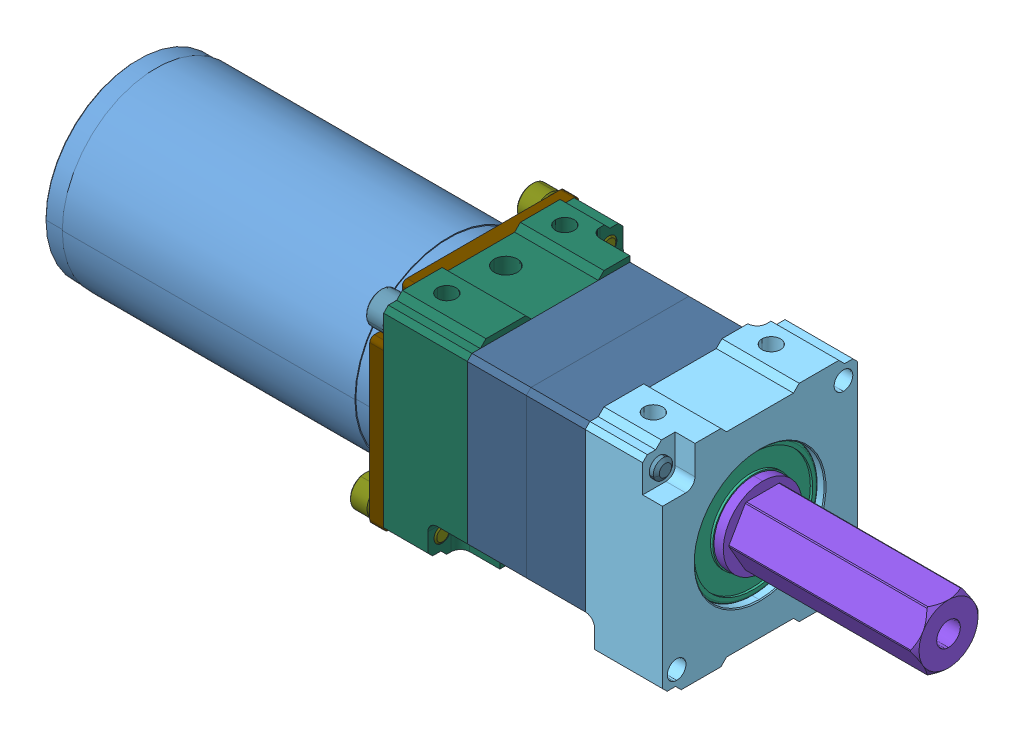
SolidWorks assembly VersaPlanetary v2 Two Stage 100_1 with BAG , configuration Default. Lengths in mm.
Overall size (176.1 66.01 66.15).
42 component instances, 19 part files, 0 mates.
Components (placement in the parent):
- VersaPlanetary v2 Two Stage 100_1 with BAG .step-1: VersaPlanetary v2 Two Stage 100_1 with BAG .step [Default] at origin size (176.1 66.01 66.15)
  - Assem5^VersaPlanetary v2 Two Stage 100_1 with BAG .step-1: Assem5^VersaPlanetary v2 Two Stage 100_1 with BAG .step [Default] at origin size (98.55 51.52 52.65) (virtual)
    - 217-2820 Rev1_Public.step-1: 217-2820 Rev1_Public.step [Default] at (-4.6546 22.225 0) x (0 -0.456494 0.889726) z (-1 0 0) size (39.22 38.88 17.4)
      - 217-2625-100.step-1: 217-2625-100.step [Default] at origin size (39.22 38.88 12.7)
        - 217-2625-008 Rev1.step-1: 217-2625-008 Rev1.step [Default] at origin size (34.7 34.7 4.7)
        - 217-2625-010 Rev1.step-1: 217-2625-010 Rev1.step [Default] at (0 10.193 3.65) x (0.999813 0.019336 0) z (0 0 1) size (4 4 12)
        - 217-2625-010 Rev1.step-2: 217-2625-010 Rev1.step [Default] at (8.691 -5.3258 3.65) size (4 4 12)
        - 217-2625-010 Rev1.step-3: 217-2625-010 Rev1.step [Default] at (-8.691 -5.3258 3.65) size (4 4 12)
        - 217-2625-005 Rev1_Planet_Revolving_Follower01.step-1: 217-2625-005 Rev1_Planet_Revolving_Follower01.step [Default] at (8.691 -5.3258 6.35) x (0.932816 0.360354 0) z (0 0 1) size (16.89 16.89 8)
        - 217-2625-005 Rev1_Planet_Revolving_Follower01.step-2: 217-2625-005 Rev1_Planet_Revolving_Follower01.step [Default] at (-8.691 -5.3258 6.35) x (-0.932788 -0.360426 0) z (0 0 1) size (16.89 16.89 8)
        - 217-2625-005 Rev1_Planet_Revolving_Follower01.step-3: 217-2625-005 Rev1_Planet_Revolving_Follower01.step [Default] at (0 10.193 6.35) x (0.893583 0.448898 0) z (0 0 1) size (16.89 16.89 8)
      - 217-2625-007 Rev1_Public.step-1: 217-2625-007 Rev1_Public.step [Default] at (0 0 6.7) x (0.992772 0.120019 0) z (0 0 1) size (15.27 15.27 12.7)
    - 217-2820 Rev1_Public.step-2: 217-2820 Rev1_Public.step [Default] at (-17.15 22.225 0) x (0 0.184082 0.982911) z (-1 0 0) size (39.22 38.88 17.4)
      - 217-2625-100.step-1: 217-2625-100.step [Default] at origin size (39.22 38.88 12.7)
        - 217-2625-008 Rev1.step-1: 217-2625-008 Rev1.step [Default] at origin size (34.7 34.7 4.7)
        - 217-2625-010 Rev1.step-1: 217-2625-010 Rev1.step [Default] at (0 10.193 3.65) x (0.999813 0.019336 0) z (0 0 1) size (4 4 12)
        - 217-2625-010 Rev1.step-2: 217-2625-010 Rev1.step [Default] at (8.691 -5.3258 3.65) size (4 4 12)
        - 217-2625-010 Rev1.step-3: 217-2625-010 Rev1.step [Default] at (-8.691 -5.3258 3.65) size (4 4 12)
        - 217-2625-005 Rev1_Planet_Revolving_Follower01.step-1: 217-2625-005 Rev1_Planet_Revolving_Follower01.step [Default] at (8.691 -5.3258 6.35) x (0.932816 0.360354 0) z (0 0 1) size (16.89 16.89 8)
        - 217-2625-005 Rev1_Planet_Revolving_Follower01.step-2: 217-2625-005 Rev1_Planet_Revolving_Follower01.step [Default] at (-8.691 -5.3258 6.35) x (-0.932788 -0.360426 0) z (0 0 1) size (16.89 16.89 8)
        - 217-2625-005 Rev1_Planet_Revolving_Follower01.step-3: 217-2625-005 Rev1_Planet_Revolving_Follower01.step [Default] at (0 10.193 6.35) x (0.893583 0.448898 0) z (0 0 1) size (16.89 16.89 8)
      - 217-2625-007 Rev1_Public.step-1: 217-2625-007 Rev1_Public.step [Default] at (0 0 6.7) x (0.992772 0.120019 0) z (0 0 1) size (15.27 15.27 12.7)
    - 217-2625-026 Rev1.step-1: 217-2625-026 Rev1.step [Default] at (-6.5 22.225 0) x (0 -1 0) z (-1 0 0) size (44.45 42 18.12)
    - 217-2742-001 Rev4.step-1: 217-2742-001 Rev4.step [Default] at (0.2002 22.225 0) x (1 0 0) z (0 -0.092627 0.995701) size (7 28 28)
    - 217-2742-001 Rev4.step-2: 217-2742-001 Rev4.step [Default] at (8.2002 22.225 0) size (7 28 28)
    - 217-2625-017 Rev1_9714K61.step-1: 217-2625-017 Rev1_9714K61.step [Default] at (7.42 22.3002 -0.342) x (0 0.56703 0.823697) z (0 -0.823697 0.56703) size (28.51 4.98 27.43)
    - 217-2625-003 Rev1.step-1: 217-2625-003 Rev1.step [Default] at (7.4478 22.225 0) x (0 -1 0) z (1 0 0) size (17 17 64.11)
    - 217-2625-018 Rev1_98541A410.step-1: 217-2625-018 Rev1_98541A410.step [Default] at (-0.7046 22.225 0) x (1 0 0) z (0 -0.017452 0.999848) size (1 19.6 17.4)
    - 217-2816-001 Rev1.step-1: 217-2816-001 Rev1.step [Default] at (-6.35 22.225 0) x (0 -1 0) z (1 0 0) size (42 42 14.51)
    - 217-2816-001 Rev1.step-2: 217-2816-001 Rev1.step [Default] at (-19.05 22.225 0) x (0 -1 0) z (1 0 0) size (42 42 14.51)
    - 217-4649-001 Rev1.step-1: 217-4649-001 Rev1.step [Default] at (-32.746 22.225 0) x (0 -1 0) z (1 0 0) size (18 18 13)
    - 217-4649-007 Rev1_94105A824.step-1: 217-4649-007 Rev1_94105A824.step [Default] at (-38.221 22.225 -6.7835) x (-0.996104 -0.088191 0) z (0 0 -1) size (4.83 4.83 4.77)
    - 217-2625-011 Rev1.step-1: 217-2625-011 Rev1.step [Default] at (-37.4818 22.225 0) x (0 0 1) z (0 -1 0) size (8.01 7.5 7.94)
  - 832-2250-Base-Kit-Screw_SSA0832-0500ZC.step-1: 832-2250-Base-Kit-Screw_SSA0832-0500ZC.step [Default] at (-43.4 4.725 -17.5) x (0 -0.767799 -0.640691) z (0 0.640691 -0.767799) size (6.73 61.21 6.73)
  - 832-2250-Base-Kit-Screw_SSA0832-0500ZC.step-2: 832-2250-Base-Kit-Screw_SSA0832-0500ZC.step [Default] at (-43.4 39.725 17.5) x (0 0.961307 0.275478) z (0 -0.275478 0.961307) size (6.73 61.21 6.73)
  - 217-2625-025 Rev1.step-1: 217-2625-025 Rev1.step [Default] at (-35.9 22.225 0) x (0 -1 0) z (-1 0 0) size (44.45 42 18)
  - 217-4649-002 Rev1_SSA0832-0500ZC.step-1: 217-4649-002 Rev1_SSA0832-0500ZC.step [Default] at (-46.4 4.2645 17.9605) x (0 0.33842 -0.940995) z (0 0.940995 0.33842) size (6.73 16.76 6.73)
  - 217-4649-002 Rev1_SSA0832-0500ZC.step-2: 217-4649-002 Rev1_SSA0832-0500ZC.step [Default] at (-46.4 40.1855 -17.9605) x (0 -0.308932 -0.951084) z (0 0.951084 -0.308932) size (6.73 16.76 6.73)
  - 217-4649-006 Rev1_SSA0004-008BA.step-1: 217-4649-006 Rev1_SSA0004-008BA.step [Default] at (-43.4 22.225 12.5) x (0 0.5 -0.866025) z (0 -0.866025 -0.5) size (7 14 7)
  - 217-4649-006 Rev1_SSA0004-008BA.step-2: 217-4649-006 Rev1_SSA0004-008BA.step [Default] at (-43.4 22.225 -12.5) x (0 -0.5 0.866025) z (0 0.866025 0.5) size (7 14 7)
  - 217-2822-003 Rev4.step-1: 217-2822-003 Rev4.step [Default] at (-44.9 22.225 0) x (0 -1 0) z (-1 0 0) size (42 42 4.8)
  - 217-3351 Rev2.step-1: 217-3351 Rev2.step [Default] at (-46.4 22.225 0) x (0 0 1) z (1 0 0) size (59.07 59.07 84.5)
